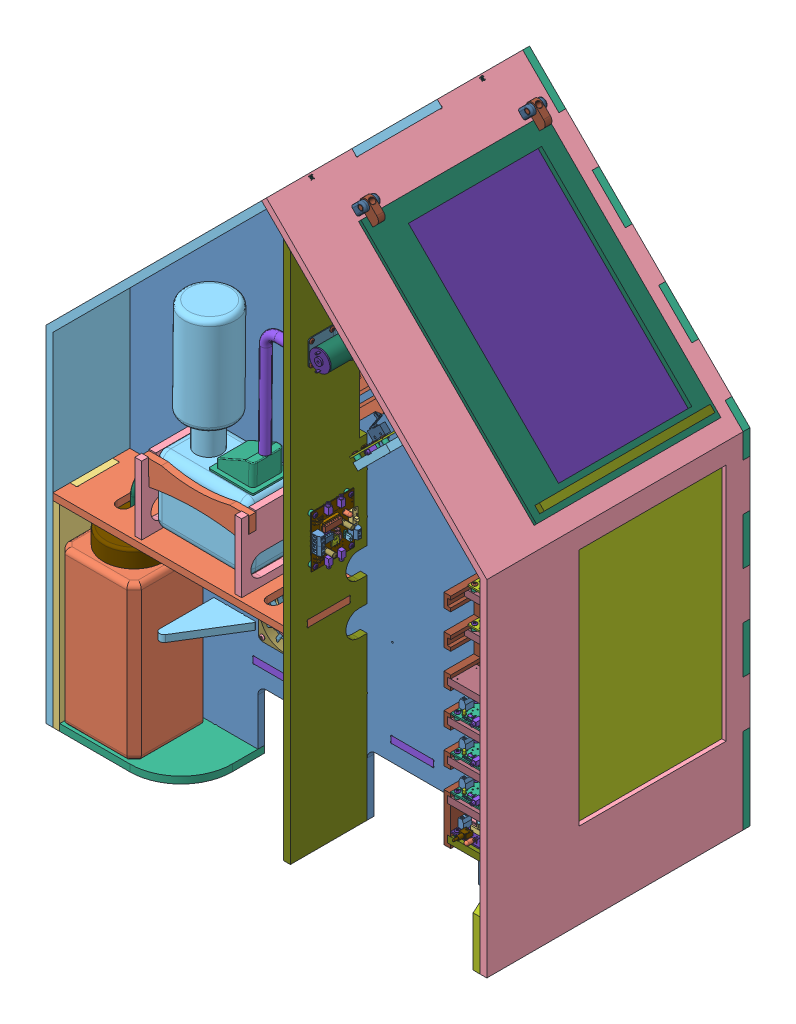
SolidWorks assembly Serre Toutes Options, configuration OLED. Lengths in mm.
Overall size (516 661.85 314.79).
495 component instances, 116 part files, 199 mates.
Components (placement in the parent):
- FONDINTERIEUR-1: FONDINTERIEUR [Défaut] at (-62.876 -300.5478 -4)
- Crémallière M3-3-1: Crémallière M3-3 [Défaut] at (-39.5374 94.1308 4) x (0.707107 0.707107 0) z (0 0 1)
- Rondelle métal 3 x 12-1: Rondelle métal 3 x 12 [Défaut] at (57.939 191.6778 8)
- VIs TC 3 x 13-1: VIs TC 3 x 13 [Défaut] at (57.939 191.6778 2.4) x (1 0 0) z (0 -1 0)
- VIs TC 3 x 13-2: VIs TC 3 x 13 [Défaut] at (22.5836 156.3225 2.4) x (1 0 0) z (0 -1 0)
- Rondelle métal 3 x 12-2: Rondelle métal 3 x 12 [Défaut] at (22.5836 156.3225 8)
- Prépa 06 module Microrupteur-1: Prépa 06 module Microrupteur [Défaut] at (80.8247 148.8026 12.3834) x (0.707107 0.707107 0) z (-0.707107 0.707107 0) size (54 40.91 95.89)
  - support capteur-1: support capteur [Défaut] at (85.4284 22.7312 -4) size (54 38 8)
  - Entretoise CI-1: Entretoise CI [Défaut] at (-25.3985 -17.6166 4) size (5.9 5.9 4.1)
  - Entretoise CI-2: Entretoise CI [Défaut] at (-25.3985 4.3834 4) size (5.9 5.9 4.1)
  - Entretoise CI-3: Entretoise CI [Défaut] at (20.6015 -17.6166 4) size (5.9 5.9 4.1)
  - Entretoise CI-4: Entretoise CI [Défaut] at (20.6015 4.3834 4) size (5.9 5.9 4.1)
  - Module Microrupteur K-AP-MMR-1: Module Microrupteur K-AP-MMR [Défaut] at (24.602 -8.2581 10.6485) x (0 1 0) z (1 0 0) size (32.91 28.24 54)
    - CI-AP-MLBP avec jack-1: CI-AP-MLBP avec jack [Défaut] at (1.5279 -1.3102 0) size (32.91 8.01 54)
      - CI BP et DEL-1: CI BP et DEL [Défaut] at (-14.8869 -1.2382 0) size (30 1.6 54)
      - Embase jack 2.5-1: Embase jack 2.5 [Défaut] at (-14.8868 -1.2382 -27.0002) x (1 0 0) z (0 0 -1) size (10.81 8.01 5)
    - Résistance 10 K pas 11-1: Résistance 10 K pas 11 [Défaut] at (-6.8591 0.4515 -37.4997) x (0 0 -1) z (1 0 0) size (11.5 4.15 2.3)
    - Microrupteur-1: Microrupteur [Défaut] at (16.351 0.0515 -46.78) x (-1 0 0) z (0 0 -1) size (6.3 24.64 22.46)
  - VIs TC 3 x 6.5-1: VIs TC 3 x 6.5 [Défaut] at (-25.3985 -17.6166 3.3) x (1 0 0) z (0 -1 0) size (5.6 8.09 5.6)
  - VIs TC 3 x 6.5-2: VIs TC 3 x 6.5 [Défaut] at (-25.3979 4.3824 3.3) x (1 0 0) z (0 -1 0) size (5.6 8.09 5.6)
  - VIs TC 3 x 6.5-3: VIs TC 3 x 6.5 [Défaut] at (20.6015 -17.6166 3.3) x (0.418214 0.908348 0) z (0.908348 -0.418214 0) size (5.6 8.09 5.6)
  - VIs TC 3 x 6.5-4: VIs TC 3 x 6.5 [Défaut] at (20.6015 4.3834 3.3) x (1 0 0) z (0 -1 0) size (5.6 8.09 5.6)
- Prépa 06 module Microrupteur-2: Prépa 06 module Microrupteur [Défaut] at (10.114 78.0919 12.3834) x (0.707107 0.707107 0) z (-0.707107 0.707107 0) size (54 40.91 95.89)
  - support capteur-1: support capteur [Défaut] at (85.4284 22.7312 -4) size (54 38 8)
  - Entretoise CI-1: Entretoise CI [Défaut] at (-25.3985 -17.6166 4) size (5.9 5.9 4.1)
  - Entretoise CI-2: Entretoise CI [Défaut] at (-25.3985 4.3834 4) size (5.9 5.9 4.1)
  - Entretoise CI-3: Entretoise CI [Défaut] at (20.6015 -17.6166 4) size (5.9 5.9 4.1)
  - Entretoise CI-4: Entretoise CI [Défaut] at (20.6015 4.3834 4) size (5.9 5.9 4.1)
  - Module Microrupteur K-AP-MMR-1: Module Microrupteur K-AP-MMR [Défaut] at (24.602 -8.2581 10.6485) x (0 1 0) z (1 0 0) size (32.91 28.24 54)
    - CI-AP-MLBP avec jack-1: CI-AP-MLBP avec jack [Défaut] at (1.5279 -1.3102 0) size (32.91 8.01 54)
      - CI BP et DEL-1: CI BP et DEL [Défaut] at (-14.8869 -1.2382 0) size (30 1.6 54)
      - Embase jack 2.5-1: Embase jack 2.5 [Défaut] at (-14.8868 -1.2382 -27.0002) x (1 0 0) z (0 0 -1) size (10.81 8.01 5)
    - Résistance 10 K pas 11-1: Résistance 10 K pas 11 [Défaut] at (-6.8591 0.4515 -37.4997) x (0 0 -1) z (1 0 0) size (11.5 4.15 2.3)
    - Microrupteur-1: Microrupteur [Défaut] at (16.351 0.0515 -46.78) x (-1 0 0) z (0 0 -1) size (6.3 24.64 22.46)
  - VIs TC 3 x 6.5-1: VIs TC 3 x 6.5 [Défaut] at (-25.3985 -17.6166 3.3) x (1 0 0) z (0 -1 0) size (5.6 8.09 5.6)
  - VIs TC 3 x 6.5-2: VIs TC 3 x 6.5 [Défaut] at (-25.3979 4.3824 3.3) x (1 0 0) z (0 -1 0) size (5.6 8.09 5.6)
  - VIs TC 3 x 6.5-3: VIs TC 3 x 6.5 [Défaut] at (20.6015 -17.6166 3.3) x (0.418214 0.908348 0) z (0.908348 -0.418214 0) size (5.6 8.09 5.6)
  - VIs TC 3 x 6.5-4: VIs TC 3 x 6.5 [Défaut] at (20.6015 4.3834 3.3) x (1 0 0) z (0 -1 0) size (5.6 8.09 5.6)
- Ventilateur-1: Ventilateur [Défaut] at (-116.5864 -162.967 9.2) size (60 60 10.4)
  - Cage ventilateur-1: Cage ventilateur [Défaut] at (-27.2896 -30.9986 -5.2) size (60 60 10.4)
  - Hélice-1: Hélice [Défaut] at (3.0209 -0.9986 1.3) x (1 0 0) z (0 -1 0) size (55.32 5 55.41)
    - centre hélice-1: centre hélice [Défaut] at (-0.3105 -2.5 0) size (28.6 5 28.6)
    - Pale-1: Pale [Défaut] at (12.924 -1.982 -2.4379) x (-0.128403 0.431224 -0.893061) z (-0.06137 -0.902245 -0.426835) size (5.38 14.29 1.25)
    - Pale-12: Pale [Défaut] at (12.1411 -1.982 5.1043) x (0.374806 0.431224 -0.820711) z (0.179137 -0.902245 -0.392255) size (5.38 14.29 1.25)
    - Pale-13: Pale [Défaut] at (7.4049 -1.982 11.0258) x (0.759017 0.431224 -0.48779) z (0.362769 -0.902245 -0.233137) size (5.38 14.29 1.25)
    - Pale-14: Pale [Défaut] at (0.2191 -1.982 13.4468) x (0.902245 0.431224 0) z (0.431224 -0.902245 0) size (5.38 14.29 1.25)
    - Pale-15: Pale [Défaut] at (-7.1349 -1.982 11.5985) x (0.759017 0.431224 0.48779) z (0.362769 -0.902245 0.233137) size (5.38 14.29 1.25)
    - Pale-16: Pale [Défaut] at (-12.3221 -1.982 6.0677) x (0.374806 0.431224 0.820711) z (0.179137 -0.902245 0.392255) size (5.38 14.29 1.25)
    - Pale-17: Pale [Défaut] at (-13.6958 -1.982 -1.3895) x (-0.128403 0.431224 0.893061) z (-0.06137 -0.902245 0.426835) size (5.38 14.29 1.25)
    - Pale-18: Pale [Défaut] at (-10.8197 -1.982 -8.4055) x (-0.590845 0.431224 0.681871) z (-0.282392 -0.902245 0.325897) size (5.38 14.29 1.25)
    - Pale-19: Pale [Défaut] at (-4.6071 -1.982 -12.7529) x (-0.865698 0.431224 0.254192) z (-0.413756 -0.902245 0.12149) size (5.38 14.29 1.25)
    - Pale-20: Pale [Défaut] at (2.9697 -1.982 -13.0513) x (-0.865698 0.431224 -0.254192) z (-0.413756 -0.902245 -0.12149) size (5.38 14.29 1.25)
    - Pale-21: Pale [Défaut] at (9.505 -1.982 -9.206) x (-0.590845 0.431224 -0.681871) z (-0.282392 -0.902245 -0.325897) size (5.38 14.29 1.25)
- VIs TC 3 x 13-4: VIs TC 3 x 13 [Défaut] at (-138.876 -138.9656 8) x (1 0 0) z (0 -1 0)
- VIs TC 3 x 13-6: VIs TC 3 x 13 [Défaut] at (-88.876 -138.9656 8) x (1 0 0) z (0 -1 0)
- VIs TC 3 x 13-7: VIs TC 3 x 13 [Défaut] at (-88.876 -188.9656 8) x (1 0 0) z (0 -1 0)
- VIs TC 3 x 13-8: VIs TC 3 x 13 [Défaut] at (-138.876 -188.9656 8) x (1 0 0) z (0 -1 0)
- Entretoise CI-1: Entretoise CI [Défaut] at (57.939 191.6778 4) x (-0.97677 0.214292 0) z (0 0 1) size (5.9 5.9 4.1)
- Entretoise CI-2: Entretoise CI [Défaut] at (22.5836 156.3225 4) size (5.9 5.9 4.1)
- VIS TORCX TF 3 X 19-1: VIS TORCX TF 3 X 19 [Défaut] at (79.1287 147.1066 -4) x (-0.923728 -0.383049 0) z (0 0 -1)
- VIS TORCX TF 3 X 19-2: VIS TORCX TF 3 X 19 [Défaut] at (8.418 76.3959 -4) x (-0.923728 -0.383049 0) z (0 0 -1)
- Prépa 02 renfort arrière-1: Prépa 02 renfort arrière [Défaut] at (-30.876 -5.636 -123.7404) x (0 0 -1) z (1 0 0) size (157.27 630.07 217.21)
  - renfortarriere-1: renfortarriere [Défaut] at (-133.6202 -294.9118 -4) size (98 630.07 8)
  - Entretoise CI-1: Entretoise CI [Défaut] at (-194.2138 26.8323 4) size (5.9 5.9 4.1)
  - Entretoise CI-2: Entretoise CI [Défaut] at (-152.2157 27.0837 4) size (5.9 5.9 4.1)
  - Entretoise CI-3: Entretoise CI [Défaut] at (-193.9025 -25.1656 4) size (5.9 5.9 4.1)
  - Entretoise CI-4: Entretoise CI [Défaut] at (-151.9044 -24.9142 4) size (5.9 5.9 4.1)
  - VIs TC 3 x 9-1: VIs TC 3 x 9 [Défaut] at (-194.2138 26.8323 2.7) x (1 0 0) z (0 -1 0) size (5.6 10.69 5.6)
  - VIs TC 3 x 9-2: VIs TC 3 x 9 [Défaut] at (-152.2157 27.0837 2.7) x (1 0 0) z (0 -1 0) size (5.6 10.69 5.6)
  - VIs TC 3 x 9-3: VIs TC 3 x 9 [Défaut] at (-151.9044 -24.9142 2.7) x (1 0 0) z (0 -1 0) size (5.6 10.69 5.6)
  - VIs TC 3 x 9-4: VIs TC 3 x 9 [Défaut] at (-193.9025 -25.1656 2.7) x (1 0 0) z (0 -1 0) size (5.6 10.69 5.6)
  - Module 2 moteurs K-AP-MMOT-1: Module 2 moteurs K-AP-MMOT [Défaut] at (-148.0718 3.1444 10.7771) x (-0.005986 0.999982 0) z (0.999982 0.005986 0) size (65.82 19.5 50.56)
    - CI moteur-1: CI moteur [Défaut] at (-32.0357 -2.6771 0) size (60 1 50)
    - BORNIER 2-1: BORNIER 2 [Default] at (-17.0423 -1.6771 0.2294) x (0.999982 0 0.005986) z (0 1 0) size (9.97 7.55 15.02)
    - DEL D5 R-1: DEL D5 R [Défaut] at (9.6889 6.8229 -10.9906) x (1 0 0) z (0 -1 0) size (5.3 5.6 11.5)
    - Embase jack 2.5-1: Embase jack 2.5 [Défaut] at (-32.0356 -1.6771 -17.5006) size (10.81 8.01 5)
    - MICRO INVERSEUR A GLISSIERE-1: MICRO INVERSEUR A GLISSIERE [Défaut] at (3.55 3.3429 -4.0189) x (1 0 0.000537) z (0 1 0) size (19 5.82 12.15)
    - Résistance 220 ohm pas 11-1: Résistance 220 ohm pas 11 [Défaut] at (-10.0359 0.3229 -18.1991) x (-1 0 0) z (0 0 -1) size (11.5 4.15 2.3)
    - Embase jack 2.5-2: Embase jack 2.5 [Défaut] at (-32.0356 -1.6771 -32.5018) size (10.81 8.01 5)
    - Embase jack 2.5-3: Embase jack 2.5 [Défaut] at (27.964 -1.6771 -17.4981) x (-1 0 0) z (0 0 -1) size (10.81 8.01 5)
    - Embase jack 2.5-4: Embase jack 2.5 [Défaut] at (27.964 -1.6771 -32.4993) x (-1 0 0) z (0 0 -1) size (10.81 8.01 5)
    - Capuchon picot-1: Capuchon picot [Défaut] at (-16.1457 0.4729 -12.7155) x (1 0 0) z (0 -1 0) size (5.05 2.51 6.1)
    - ASB 3PICOTS-1: ASB 3PICOTS [Default] at (-9.9569 2.4259 -10.7946) x (1 0 0) z (0 -1 0) size (7.59 2.51 10)
      - PICOT-1: PICOT [Default] at (26.8516 -23.7306 1.953) size (2.51 2.51 10)
      - PICOT-2: PICOT [Default] at (29.3916 -23.7306 1.953) size (2.51 2.51 10)
      - PICOT-3: PICOT [Default] at (24.3116 -23.7306 1.953) size (2.51 2.51 10)
    - AJUSTABLE H-1: AJUSTABLE H [Défaut] at (-15.4716 0.3229 -24.988) x (0 0 1) z (0 1 0) size (8.6 10.76 7.4)
    - BORNIER 2-2: BORNIER 2 [Default] at (-2.0505 -1.6771 -50.2748) x (-1 0 0) z (0 1 0) size (9.97 7.55 15.02)
    - BORNIER 2-3: BORNIER 2 [Default] at (7.9495 -1.6771 -50.2748) x (-1 0 0) z (0 1 0) size (9.97 7.55 15.02)
    - Résistance 10 K pas 11-1: Résistance 10 K pas 11 [Défaut] at (19.1656 0.3229 -42.727) x (0 0 -1) z (1 0 0) size (11.5 4.15 2.3)
    - Résistance 10 K pas 11-2: Résistance 10 K pas 11 [Défaut] at (15.6274 0.3229 -42.6914) x (0 0 -1) z (1 0 0) size (11.5 4.15 2.3)
    - Résistance 10 K pas 11-3: Résistance 10 K pas 11 [Défaut] at (-19.5364 0.3229 -42.0005) x (0 0 -1) z (1 0 0) size (11.5 4.15 2.3)
    - Résistance 10 K pas 11-4: Résistance 10 K pas 11 [Défaut] at (-23.0365 0.3229 -42.0005) x (0 0 -1) z (1 0 0) size (11.5 4.15 2.3)
    - Support CI 8 pattes-1: Support CI 8 pattes [Défaut] at (-2.7368 -1.6771 -30.0083) x (0 0 -1) z (1 0 0) size (10 6 10.1)
    - Support CI 16 pattes-1: Support CI 16 pattes [Défaut] at (8.6068 -1.6771 -19.8458) x (0 0 -1) z (1 0 0) size (20.1 6 10.1)
    - CI 8 pattes-1: CI 8 pattes [Défaut] at (-2.7368 1.3229 -30.0113) x (0 0 -1) z (1 0 0) size (10 7.2 7.8)
    - CI 16 pattes-1: CI 16 pattes [Défaut] at (8.6068 1.3229 -19.8488) x (0 0 -1) z (1 0 0) size (20.1 7.2 7.8)
    - Capa 16V 100F 2.54-1: Capa 16V 100F 2.54 [Default] at (-14.0347 -26.6935 -37.5006) x (0 0 1) z (-1 0 0) size (5.2 15.5 5.88)
    - Capa 16V 100F 2.54-2: Capa 16V 100F 2.54 [Default] at (2.9618 -26.6935 -15.9995) x (0.999999 0 0.001464) z (-0.001464 0 0.999999) size (5.2 15.5 5.88)
    - condensateur 100nF-1: condensateur 100nF [Default] at (-2.9304 -7.4359 -15.4031) x (0 0 -1) z (1 0 0) size (5.85 10.35 1.99)
    - condensateur 100nF-2: condensateur 100nF [Default] at (0.5738 -7.4359 -15.3738) x (0 0 -1) z (1 0 0) size (5.85 10.35 1.99)
  - Moteur MFA 12-24V-1: Moteur MFA 12-24V [Défaut] at (-181.5572 189.3895 16.5047) x (-1 0 0) z (0 1 0) size (70.4 27.9 30)
    - Support moteur-1: Support moteur [Défaut] at (-14.3868 -12.5047 0) size (31 26.4 30)
    - Corps moteur-1: Corps moteur [Défaut] at (14.8132 1.8953 0) x (0 0 1) z (-1 0 0) size (24 24 63.9)
    - Capuchon moteur-1: Capuchon moteur [Défaut] at (-15.3868 1.8953 0) x (0 0 1) z (-1 0 0) size (27 27 18.7)
    - Arrière moteur-1: Arrière moteur [Défaut] at (16.3132 1.8953 0) x (0 0 1) z (-1 0 0) size (24 24 6.5)
  - Prépa 01 roue dentée-1: Prépa 01 roue dentée [Défaut] at (-131.9704 192.8178 10.3013) x (0 0.156764 -0.987636) z (1 0 0) size (54 54 71.42)
    - roue dentée 16-1: roue dentée 16 [Défaut] at (-7.1573 -1.556 -4) size (54 54 8)
    - Bague d'arrêt 4x12x24-1: Bague d'arrêt 4x12x24 [Défaut] at (-8.536 -2.1164 -10) x (0 1 0) z (0 0 1) size (24 24 8)
    - VIs TC 3 x 6.5-1: VIs TC 3 x 6.5 [Défaut] at (-8.536 6.8836 2.4) x (1 0 0) z (0 1 0) size (5.6 8.09 5.6)
    - VIs TC 3 x 6.5-2: VIs TC 3 x 6.5 [Défaut] at (-8.536 -11.1164 2.4) x (1 0 0) z (0 1 0) size (5.6 8.09 5.6)
  - VIs TC 3 x 6.5-1: VIs TC 3 x 6.5 [Défaut] at (-194.1704 201.3895 -1.4) x (1 0 0) z (0 -1 0) size (5.6 8.09 5.6)
  - VIs TC 3 x 6.5-2: VIs TC 3 x 6.5 [Défaut] at (-170.1704 201.3895 -1.4) x (1 0 0) z (0 -1 0) size (5.6 8.09 5.6)
  - VIs TC 3 x 6.5-3: VIs TC 3 x 6.5 [Défaut] at (-194.1704 177.3895 -1.4) x (1 0 0) z (0 -1 0) size (5.6 8.09 5.6)
  - VIs TC 3 x 6.5-4: VIs TC 3 x 6.5 [Défaut] at (-170.1704 177.3895 -1.4) x (1 0 0) z (0 -1 0) size (5.6 8.09 5.6)
- étagèrebrumi-1: étagèrebrumi [Défaut] at (-62.876 -93.9656 245.3364) x (1 0 0) z (0 1 0)
- VIS TORCX TF 3 X 19-3: VIS TORCX TF 3 X 19 [Défaut] at (-30.876 -315.9656 -4) x (-0.991079 -0.133274 0) z (0 0 -1)
- VIS TORCX TF 3 X 19-4: VIS TORCX TF 3 X 19 [Défaut] at (-30.876 -274.5499 -4) x (-0.991079 -0.133274 0) z (0 0 -1)
- VIS TORCX TF 3 X 19-5: VIS TORCX TF 3 X 19 [Défaut] at (-169.876 -89.9656 -4) x (-0.991079 -0.133274 0) z (0 0 -1)
- VIS TORCX TF 3 X 19-6: VIS TORCX TF 3 X 19 [Défaut] at (-30.876 -27.0369 -4) x (-0.991079 -0.133274 0) z (0 0 -1)
- VIS TORCX TF 3 X 19-7: VIS TORCX TF 3 X 19 [Défaut] at (-30.876 278.5344 -4) x (-0.991079 -0.133274 0) z (0 0 -1)
- Coté gauche serre-1: Coté gauche serre [Défaut] at (-304.876 -288.0405 43.9648) x (0 0 -1) z (1 0 0)
- Coté support brumisateur-1: Coté support brumisateur [Défaut] at (-87.876 -76.5368 52.2063) x (0 0 1) z (-1 0 0)
- Coté support brumisateur-2: Coté support brumisateur [Défaut] at (-204.876 -76.5368 52.2063) x (0 0 1) z (-1 0 0)
- Renfort bidon-1: Renfort bidon [Défaut] at (-206.376 -195.9656 85) x (1 0 0) z (0 1 0)
- suportbloceau-1: suportbloceau [Défaut] at (-238.3888 -323.9656 72.4161) x (1 0 0) z (0 1 0)
- VIS TORCX TF 3 X 19-12: VIS TORCX TF 3 X 19 [Défaut] at (-198.876 -191.9656 -4) x (-0.923728 -0.383049 0) z (0 0 -1)
- VIS TORCX TF 3 X 19-13: VIS TORCX TF 3 X 19 [Défaut] at (-164.4919 -191.9656 -4) x (-0.923728 -0.383049 0) z (0 0 -1)
- VIS TORCX TF 3 X 19-14: VIS TORCX TF 3 X 19 [Défaut] at (-208.876 -75.9656 -4) x (-0.923728 -0.383049 0) z (0 0 -1)
- VIS TORCX TF 3 X 19-15: VIS TORCX TF 3 X 19 [Défaut] at (-208.876 -16.4656 -4) x (-0.923728 -0.383049 0) z (0 0 -1)
- VIS TORCX TF 3 X 19-16: VIS TORCX TF 3 X 19 [Défaut] at (-91.876 -75.9656 -4) x (-0.923728 -0.383049 0) z (0 0 -1)
- VIS TORCX TF 3 X 19-17: VIS TORCX TF 3 X 19 [Défaut] at (-91.876 -15.9656 -4) x (-0.923728 -0.383049 0) z (0 0 -1)
- VIS TORCX TF 3 X 19-18: VIS TORCX TF 3 X 19 [Défaut] at (-304.876 -89.9656 48.9996) x (0 0 1) z (-1 0 0)
- VIS TORCX TF 3 X 19-25: VIS TORCX TF 3 X 19 [Défaut] at (-304.876 -248.9656 -0.0009) x (0 0 1) z (-1 0 0)
- VIS TORCX TF 3 X 19-26: VIS TORCX TF 3 X 19 [Défaut] at (-300.876 -323.9656 49) x (0.782535 0 -0.622606) z (0 -1 0)
- VIS TORCX TF 3 X 19-29: VIS TORCX TF 3 X 19 [Défaut] at (-271.876 -323.9656 0) x (0.782535 0 -0.622606) z (0 -1 0)
- VIS TORCX TF 3 X 19-30: VIS TORCX TF 3 X 19 [Défaut] at (-179.876 -323.9656 0) x (0.782535 0 -0.622606) z (0 -1 0)
- Coté droit serre-1: Coté droit serre [Défaut] at (187.124 -288.4466 43.9657) x (0 0 -1) z (1 0 0)
- VIS TORCX TF 3 X 19-35: VIS TORCX TF 3 X 19 [Défaut] at (195.124 -248.9656 0) x (0 -0.192039 -0.981387) z (1 0 0)
- Poutre fond-1: Poutre fond [Défaut] at (-62.876 -231.9656 64.5822) x (1 0 0) z (0 1 0)
- VIS TORCX TF 3 X 19-36: VIS TORCX TF 3 X 19 [Défaut] at (-213.1345 -227.9656 4)
- VIS TORCX TF 3 X 19-37: VIS TORCX TF 3 X 19 [Défaut] at (-54.876 -227.9656 4)
- Poutre plateau-1: Poutre plateau [Défaut] at (79.7388 -229.6404 -13) x (-1 0 0) z (0 0 -1)
- façadeporteplateau-1: façadeporteplateau [Défaut] at (102.5126 -276.3164 -206)
- VIS TORCX TF 3 X 19-38: VIS TORCX TF 3 X 19 [Défaut] at (191.124 -273.9656 -206) x (-0.923728 -0.383049 0) z (0 0 -1)
- VIS TORCX TF 3 X 19-39: VIS TORCX TF 3 X 19 [Défaut] at (195.124 -308.9656 -202) x (0 0 -1) z (1 0 0)
- VIS TORCX TF 3 X 19-40: VIS TORCX TF 3 X 19 [Défaut] at (195.124 -238.9656 -202) x (0 0 -1) z (1 0 0)
- VIS TORCX TF 3 X 19-43: VIS TORCX TF 3 X 19 [Défaut] at (-300.876 -273.9656 -206) x (-0.923728 -0.383049 0) z (0 0 -1)
- VIS TORCX TF 3 X 19-44: VIS TORCX TF 3 X 19 [Défaut] at (-304.876 -238.9737 -202) x (0 0 1) z (-1 0 0)
- VIS TORCX TF 3 X 19-45: VIS TORCX TF 3 X 19 [Défaut] at (-304.876 -308.9656 -202) x (0 0 1) z (-1 0 0)
- VIS TORCX TF 3 X 19-49: VIS TORCX TF 3 X 19 [Défaut] at (103.3825 -227.9656 4)
- Sous ensemble Rack module Toutes Options-1: Sous ensemble Rack module Toutes Options [Défaut] at (116.8547 -126.3174 -67.6389) x (0 0 -1) z (1 0 0) size (72.22 263.1 70)
  - rack coté gauche-1: rack coté gauche [Défaut] at (-102.2159 -95.6801 -4) size (58 256 8)
  - rack coté droit-1: rack coté droit [Défaut] at (-102.2159 -95.6628 58) size (58 256 8)
  - Prépa 05 module TEMP-1: Prépa 05 module TEMP [Défaut] at (-82.7846 122.513 33.0896) x (0 0 1) z (0 1 0) size (62 41.41 95.55)
    - supportcarterack-1: supportcarterack [Défaut] at (3.5074 9.0286 -6.1612) size (62 30 8)
    - Entretoise CI-1: Entretoise CI [Défaut] at (-25.0896 -14.8542 1.8388) size (5.9 5.9 4.1)
    - Entretoise CI-2: Entretoise CI [Défaut] at (-25.0896 7.1458 1.8388) size (5.9 5.9 4.1)
    - Entretoise CI-3: Entretoise CI [Défaut] at (20.9104 -14.8542 1.8388) size (5.9 5.9 4.1)
    - Entretoise CI-4: Entretoise CI [Défaut] at (20.9104 7.1458 1.8388) size (5.9 5.9 4.1)
    - Module temperature K-AP-MTEMP-1: Module temperature K-AP-MTEMP [Défaut] at (24.9109 -3.9678 7.1771) x (0 1 0) z (1 0 0) size (41.41 8.39 54)
      - CI BP et DEL-1: CI BP et DEL [Défaut] at (-14.8869 -1.2382 0) size (30 1.6 54)
      - Embase jack 2.5-1: Embase jack 2.5 [Défaut] at (-14.8868 0.3618 -27.0002) size (10.81 8.01 5)
      - Résistance 3,9 K pas 11-1: Résistance 3,9 K pas 11 [Défaut] at (-12.3875 1.7618 -37.4997) x (0 0 1) z (-1 0 0) size (11.5 4.15 2.3)
      - RC1 Tansistor plié 90°-1: RC1 Tansistor plié 90° [Défaut] at (18.6119 3.3399 -22.4989) x (0 0 -1) z (0 -1 0) size (4.8 10.25 6.98)
    - VIs TC 3 x 6.5-1: VIs TC 3 x 6.5 [Défaut] at (-25.0896 -14.8542 1.1388) x (1 0 0) z (0 -1 0) size (5.6 8.09 5.6)
    - VIs TC 3 x 6.5-2: VIs TC 3 x 6.5 [Défaut] at (-25.0896 7.1458 1.1388) x (1 0 0) z (0 -1 0) size (5.6 8.09 5.6)
    - VIs TC 3 x 6.5-3: VIs TC 3 x 6.5 [Défaut] at (20.9104 7.1458 1.1388) x (1 0 0) z (0 -1 0) size (5.6 8.09 5.6)
    - VIs TC 3 x 6.5-4: VIs TC 3 x 6.5 [Défaut] at (20.9104 -14.8542 1.1388) x (1 0 0) z (0 -1 0) size (5.6 8.09 5.6)
  - VIS TORCX TF 3 X 19-1: VIS TORCX TF 3 X 19 [Défaut] at (-86.6389 120.3518 66)
  - VIS TORCX TF 3 X 19-2: VIS TORCX TF 3 X 19 [Défaut] at (-86.6389 120.3431 -4) x (-0.923728 -0.383049 0) z (0 0 -1)
  - Prépa 04 module MAFU-1: Prépa 04 module MAFU [Défaut] at (-94.8752 -119.6656 28.2245) x (0 0 1) z (0 1 0) size (62 61.57 131.04)
    - basesuportpuissance-1: basesuportpuissance [Défaut] at (-4.8343 -1.5394 -4) size (62 50 8)
    - Entretoise CI-1: Entretoise CI [Défaut] at (-20.2245 -22.7636 4) size (5.9 5.9 4.1)
    - Entretoise CI-2: Entretoise CI [Défaut] at (-20.2245 -0.7636 4) size (5.9 5.9 4.1)
    - Entretoise CI-3: Entretoise CI [Défaut] at (25.7755 -0.7636 4) size (5.9 5.9 4.1)
    - Entretoise CI-4: Entretoise CI [Défaut] at (25.7755 -22.7636 4) size (5.9 5.9 4.1)
    - CI-MAFU avec borniers-1: CI-MAFU avec borniers [Défaut] at (2.9088 -18.7288 8.9) x (0 -1 0) z (0 0 1) size (43.65 55.05 18.42)
      - CI-MAFU-1: CI-MAFU [Défaut] at (-21.9652 -27.1333 -0.8) size (30 54 1.6)
      - Inter long à souder 734-7220-1: Inter long à souder 734-7220 [Défaut] at (8.1051 -9.1203 1.3) x (-1 0 0) z (0 1 0) size (20.8 9.2 8)
      - Embase femelle d'alimentation-1: Embase femelle d'alimentation [Défaut] at (4.7338 12.8853 0.8) x (0 -1 0) z (-1 0 0) size (10.39 15 14.1)
      - DEL D5 rouge pliée-2: DEL D5 rouge pliée [Défaut] at (17.5325 -1.131 5.2) x (0 1 0) z (-1 0 0) size (5.3 8.8 12.9)
      - Support fusible avec fusible-1: Support fusible avec fusible [Défaut] at (-8.3615 -5.1853 4.8987) x (0 1 0) z (1 0 0) size (23 17 8.6)
        - Support fusible base-1: Support fusible base [Défaut] at (-10.9359 -4.0987 -4.3) size (22 7 8.6)
        - Support fusible contact-1: Support fusible contact [Défaut] at (5.4641 0.8731 -0.0014) size (6.1 17 6.2)
        - Support fusible contact-2: Support fusible contact [Défaut] at (-5.3359 0.8731 -0.0014) x (-1 0 0) z (0 0 -1) size (6.1 17 6.2)
        - Fusible-1: Fusible [Défaut] at (-0.0359 6.2731 -0.0014) size (19.8 5.2 5.2)
      - BORNIER 2-2: BORNIER 2 [Default] at (-24.0402 -10.1483 0.8) x (0 -1 0) z (0 0 1) size (9.97 7.55 15.02)
      - BORNIER 2-4: BORNIER 2 [Default] at (-24.0402 -0.1483 0.8) x (0 -1 0) z (0 0 1) size (9.97 7.55 15.02)
      - BORNIER 2-5: BORNIER 2 [Default] at (-24.0402 9.8517 0.8) x (0 -1 0) z (0 0 1) size (9.97 7.55 15.02)
      - BORNIER 2-6: BORNIER 2 [Default] at (-24.0402 19.8517 0.8) x (0 -1 0) z (0 0 1) size (9.97 7.55 15.02)
      - BORNIER 2-7: BORNIER 2 [Default] at (-10.2502 -27.9083 0.8) size (9.97 7.55 15.02)
      - BORNIER 2-9: BORNIER 2 [Default] at (-0.2802 27.1417 0.8) x (-1 0 0) z (0 0 1) size (9.97 7.55 15.02) (hidden)
    - VIs TC 3 x 9-1: VIs TC 3 x 9 [Défaut] at (-20.2245 -22.7636 3.3) x (1 0 0) z (0 -1 0) size (5.6 10.69 5.6)
    - VIs TC 3 x 9-2: VIs TC 3 x 9 [Défaut] at (25.7755 -22.7636 3.3) x (1 0 0) z (0 -1 0) size (5.6 10.69 5.6)
    - VIs TC 3 x 9-3: VIs TC 3 x 9 [Défaut] at (-20.2245 -0.7636 3.3) x (1 0 0) z (0 -1 0) size (5.6 10.69 5.6)
    - VIs TC 3 x 9-4: VIs TC 3 x 9 [Défaut] at (25.7755 -0.7636 3.3) x (1 0 0) z (0 -1 0) size (5.6 10.69 5.6)
  - VIS TORCX TF 3 X 19-3: VIS TORCX TF 3 X 19 [Défaut] at (-107.1389 -119.6824 66)
  - VIS TORCX TF 3 X 19-4: VIS TORCX TF 3 X 19 [Défaut] at (-78.1389 -119.6824 66)
  - VIS TORCX TF 3 X 19-6: VIS TORCX TF 3 X 19 [Défaut] at (-107.1389 -119.6656 -4) x (-0.923728 -0.383049 0) z (0 0 -1)
  - VIS TORCX TF 3 X 19-7: VIS TORCX TF 3 X 19 [Défaut] at (-78.1389 -119.6656 -4) x (-0.923728 -0.383049 0) z (0 0 -1)
  - Prépa 03 module PWR-1: Prépa 03 module PWR [Défaut] at (-104.636 -79.6656 32.1892) x (0 0 1) z (0 1 0) size (62 33.06 100.16)
    - supportcarterack-1: supportcarterack [Défaut] at (4.4079 10.88 -4) size (62 30 8)
    - Entretoise CI-1: Entretoise CI [Défaut] at (-24.1892 -13.0028 4) size (5.9 5.9 4.1)
    - Entretoise CI-2: Entretoise CI [Défaut] at (-24.1892 8.9972 4) size (5.9 5.9 4.1)
    - Entretoise CI-3: Entretoise CI [Défaut] at (21.8108 8.9972 4) size (5.9 5.9 4.1)
    - Entretoise CI-4: Entretoise CI [Défaut] at (21.8108 -13.0028 4) size (5.9 5.9 4.1)
    - Module K-AP-MPWR-1: Module K-AP-MPWR [Défaut] at (-1.2571 1.9363 8.9) x (0 1 0) z (0 0 1) size (33.06 54.47 15.02)
      - CI AP-PWR-1: CI AP-PWR [Défaut] at (-18.9391 -27.0679 -0.8) size (30 54 1.6)
      - BORNIER 2-1: BORNIER 2 [Default] at (0.963 27.1235 0.8) x (-1 0 0) z (0 0 1) size (9.97 7.55 15.02)
      - DELverte 3mm-1: DELverte 3mm [Défaut] at (-12.9358 16.93 1.8) x (0 0 1) z (-1 0 0) size (7.4 3.42 3.8)
      - diode-1: diode [Défaut] at (-12.9396 11.4315 3.2) x (1 0 0) z (0 -1 0) size (2.65 5.32 8.12)
      - ASB 3PICOTS avec capuchon-1: ASB 3PICOTS avec capuchon [Default] at (-16.084 -16.9024 4.903) x (-1 0 0) z (0 0 -1) size (7.59 2.51 10.25)
        - PICOT-1: PICOT [Default] at (26.8516 -23.7306 1.953) size (2.51 2.51 10)
        - PICOT-2: PICOT [Default] at (29.3916 -23.7306 1.953) size (2.51 2.51 10)
        - PICOT-3: PICOT [Default] at (24.3116 -23.7306 1.953) size (2.51 2.51 10)
        - Capuchon picot-1: Capuchon picot [Défaut] at (-6.1888 -1.9209 1.953) size (5.05 2.51 6.1)
      - Embase jack 2.5-1: Embase jack 2.5 [Défaut] at (-18.9403 -0.0677 0.8) x (1 0 0) z (0 -1 0) size (10.81 8.01 5)
      - REG-1: REG [Default] at (-4.2884 5.0073 0.8) x (0 -1 0) z (0 0 1) size (10.15 20.05 5.19)
      - Résistance 220 pas 11-1: Résistance 220 pas 11 [Défaut] at (-17.2386 9.3312 2.2) x (0 -1 0) z (-1 0 0) size (11.5 4.15 2.3)
      - Résistance 10K pas de 11-1: Résistance 10K pas de 11 [Défaut] at (-17.2386 -9.3683 2.2) x (0 -1 0) z (-1 0 0) size (11.5 4.15 2.3)
      - BORNIER 2-2: BORNIER 2 [Default] at (-8.9238 -27.3428 0.8) size (9.97 7.55 15.02)
    - VIs TC 3 x 9-1: VIs TC 3 x 9 [Défaut] at (-24.1892 -13.0028 3.3) x (1 0 0) z (0 -1 0) size (5.6 10.69 5.6)
    - VIs TC 3 x 9-2: VIs TC 3 x 9 [Défaut] at (-24.1892 8.9972 3.3) x (1 0 0) z (0 -1 0) size (5.6 10.69 5.6)
    - VIs TC 3 x 9-3: VIs TC 3 x 9 [Défaut] at (21.8108 8.9972 3.3) x (1 0 0) z (0 -1 0) size (5.6 10.69 5.6)
    - VIs TC 3 x 9-4: VIs TC 3 x 9 [Défaut] at (21.8108 -13.0028 3.3) x (1 0 0) z (0 -1 0) size (5.6 10.69 5.6)
  - supportcarterack-3: supportcarterack [Défaut] at (-119.5217 44.3518 36.597) x (0 0 1) z (0 -1 0) size (62 30 8)
  - Prépa 03 module PWR-2: Prépa 03 module PWR [Défaut] at (-104.636 -39.6656 32.1892) x (0 0 1) z (0 1 0) size (62 33.06 100.16)
    - supportcarterack-1: supportcarterack [Défaut] at (4.4079 10.88 -4) size (62 30 8)
    - Entretoise CI-1: Entretoise CI [Défaut] at (-24.1892 -13.0028 4) size (5.9 5.9 4.1)
    - Entretoise CI-2: Entretoise CI [Défaut] at (-24.1892 8.9972 4) size (5.9 5.9 4.1)
    - Entretoise CI-3: Entretoise CI [Défaut] at (21.8108 8.9972 4) size (5.9 5.9 4.1)
    - Entretoise CI-4: Entretoise CI [Défaut] at (21.8108 -13.0028 4) size (5.9 5.9 4.1)
    - Module K-AP-MPWR-1: Module K-AP-MPWR [Défaut] at (-1.2571 1.9363 8.9) x (0 1 0) z (0 0 1) size (33.06 54.47 15.02)
      - CI AP-PWR-1: CI AP-PWR [Défaut] at (-18.9391 -27.0679 -0.8) size (30 54 1.6)
      - BORNIER 2-1: BORNIER 2 [Default] at (0.963 27.1235 0.8) x (-1 0 0) z (0 0 1) size (9.97 7.55 15.02)
      - DELverte 3mm-1: DELverte 3mm [Défaut] at (-12.9358 16.93 1.8) x (0 0 1) z (-1 0 0) size (7.4 3.42 3.8)
      - diode-1: diode [Défaut] at (-12.9396 11.4315 3.2) x (1 0 0) z (0 -1 0) size (2.65 5.32 8.12)
      - ASB 3PICOTS avec capuchon-1: ASB 3PICOTS avec capuchon [Default] at (-16.084 -16.9024 4.903) x (-1 0 0) z (0 0 -1) size (7.59 2.51 10.25)
        - PICOT-1: PICOT [Default] at (26.8516 -23.7306 1.953) size (2.51 2.51 10)
        - PICOT-2: PICOT [Default] at (29.3916 -23.7306 1.953) size (2.51 2.51 10)
        - PICOT-3: PICOT [Default] at (24.3116 -23.7306 1.953) size (2.51 2.51 10)
        - Capuchon picot-1: Capuchon picot [Défaut] at (-6.1888 -1.9209 1.953) size (5.05 2.51 6.1)
      - Embase jack 2.5-1: Embase jack 2.5 [Défaut] at (-18.9403 -0.0677 0.8) x (1 0 0) z (0 -1 0) size (10.81 8.01 5)
      - REG-1: REG [Default] at (-4.2884 5.0073 0.8) x (0 -1 0) z (0 0 1) size (10.15 20.05 5.19)
      - Résistance 220 pas 11-1: Résistance 220 pas 11 [Défaut] at (-17.2386 9.3312 2.2) x (0 -1 0) z (-1 0 0) size (11.5 4.15 2.3)
      - Résistance 10K pas de 11-1: Résistance 10K pas de 11 [Défaut] at (-17.2386 -9.3683 2.2) x (0 -1 0) z (-1 0 0) size (11.5 4.15 2.3)
      - BORNIER 2-2: BORNIER 2 [Default] at (-8.9238 -27.3428 0.8) size (9.97 7.55 15.02)
    - VIs TC 3 x 9-1: VIs TC 3 x 9 [Défaut] at (-24.1892 -13.0028 3.3) x (1 0 0) z (0 -1 0) size (5.6 10.69 5.6)
    - VIs TC 3 x 9-2: VIs TC 3 x 9 [Défaut] at (-24.1892 8.9972 3.3) x (1 0 0) z (0 -1 0) size (5.6 10.69 5.6)
    - VIs TC 3 x 9-3: VIs TC 3 x 9 [Défaut] at (21.8108 8.9972 3.3) x (1 0 0) z (0 -1 0) size (5.6 10.69 5.6)
    - VIs TC 3 x 9-4: VIs TC 3 x 9 [Défaut] at (21.8108 -13.0028 3.3) x (1 0 0) z (0 -1 0) size (5.6 10.69 5.6)
  - Prépa 03 module PWR-3: Prépa 03 module PWR [Défaut] at (-104.636 0.3344 32.1892) x (0 0 1) z (0 1 0) size (62 33.06 100.16)
    - supportcarterack-1: supportcarterack [Défaut] at (4.4079 10.88 -4) size (62 30 8)
    - Entretoise CI-1: Entretoise CI [Défaut] at (-24.1892 -13.0028 4) size (5.9 5.9 4.1)
    - Entretoise CI-2: Entretoise CI [Défaut] at (-24.1892 8.9972 4) size (5.9 5.9 4.1)
    - Entretoise CI-3: Entretoise CI [Défaut] at (21.8108 8.9972 4) size (5.9 5.9 4.1)
    - Entretoise CI-4: Entretoise CI [Défaut] at (21.8108 -13.0028 4) size (5.9 5.9 4.1)
    - Module K-AP-MPWR-1: Module K-AP-MPWR [Défaut] at (-1.2571 1.9363 8.9) x (0 1 0) z (0 0 1) size (33.06 54.47 15.02)
      - CI AP-PWR-1: CI AP-PWR [Défaut] at (-18.9391 -27.0679 -0.8) size (30 54 1.6)
      - BORNIER 2-1: BORNIER 2 [Default] at (0.963 27.1235 0.8) x (-1 0 0) z (0 0 1) size (9.97 7.55 15.02)
      - DELverte 3mm-1: DELverte 3mm [Défaut] at (-12.9358 16.93 1.8) x (0 0 1) z (-1 0 0) size (7.4 3.42 3.8)
      - diode-1: diode [Défaut] at (-12.9396 11.4315 3.2) x (1 0 0) z (0 -1 0) size (2.65 5.32 8.12)
      - ASB 3PICOTS avec capuchon-1: ASB 3PICOTS avec capuchon [Default] at (-16.084 -16.9024 4.903) x (-1 0 0) z (0 0 -1) size (7.59 2.51 10.25)
        - PICOT-1: PICOT [Default] at (26.8516 -23.7306 1.953) size (2.51 2.51 10)
        - PICOT-2: PICOT [Default] at (29.3916 -23.7306 1.953) size (2.51 2.51 10)
        - PICOT-3: PICOT [Default] at (24.3116 -23.7306 1.953) size (2.51 2.51 10)
        - Capuchon picot-1: Capuchon picot [Défaut] at (-6.1888 -1.9209 1.953) size (5.05 2.51 6.1)
      - Embase jack 2.5-1: Embase jack 2.5 [Défaut] at (-18.9403 -0.0677 0.8) x (1 0 0) z (0 -1 0) size (10.81 8.01 5)
      - REG-1: REG [Default] at (-4.2884 5.0073 0.8) x (0 -1 0) z (0 0 1) size (10.15 20.05 5.19)
      - Résistance 220 pas 11-1: Résistance 220 pas 11 [Défaut] at (-17.2386 9.3312 2.2) x (0 -1 0) z (-1 0 0) size (11.5 4.15 2.3)
      - Résistance 10K pas de 11-1: Résistance 10K pas de 11 [Défaut] at (-17.2386 -9.3683 2.2) x (0 -1 0) z (-1 0 0) size (11.5 4.15 2.3)
      - BORNIER 2-2: BORNIER 2 [Default] at (-8.9238 -27.3428 0.8) size (9.97 7.55 15.02)
    - VIs TC 3 x 9-1: VIs TC 3 x 9 [Défaut] at (-24.1892 -13.0028 3.3) x (1 0 0) z (0 -1 0) size (5.6 10.69 5.6)
    - VIs TC 3 x 9-2: VIs TC 3 x 9 [Défaut] at (-24.1892 8.9972 3.3) x (1 0 0) z (0 -1 0) size (5.6 10.69 5.6)
    - VIs TC 3 x 9-3: VIs TC 3 x 9 [Défaut] at (21.8108 8.9972 3.3) x (1 0 0) z (0 -1 0) size (5.6 10.69 5.6)
    - VIs TC 3 x 9-4: VIs TC 3 x 9 [Défaut] at (21.8108 -13.0028 3.3) x (1 0 0) z (0 -1 0) size (5.6 10.69 5.6)
  - Prépa 07 module Humidité-1: Prépa 07 module Humidité [Défaut] at (-82.3194 80.3344 31.1565) x (0 0 1) z (0 1 0) size (62 43.56 18.7)
    - supportcarterack-1: supportcarterack [Défaut] at (5.4405 8.5634 -4) size (62 30 8)
    - Entretoise CI-1: Entretoise CI [Défaut] at (-23.1565 -15.3194 4) size (5.9 5.9 4.1)
    - Entretoise CI-2: Entretoise CI [Défaut] at (-23.1565 6.6806 4) size (5.9 5.9 4.1)
    - Entretoise CI-3: Entretoise CI [Défaut] at (22.8435 -15.3194 4) size (5.9 5.9 4.1)
    - Entretoise CI-4: Entretoise CI [Défaut] at (22.8435 6.6806 4) size (5.9 5.9 4.1)
    - Carte M-HUM-1: Carte M-HUM [Défaut] at (26.844 -4.433 9.3382) x (0 1 0) z (1 0 0) size (43.56 8.01 54)
      - CI BP et DEL-1: CI BP et DEL [Défaut] at (-14.8869 -1.2382 0) size (30 1.6 54)
      - Embase jack 2.5-1: Embase jack 2.5 [Défaut] at (-14.8868 0.3618 -27.0002) size (10.81 8.01 5)
      - Résistance 150 k pas 11-1: Résistance 150 k pas 11 [Défaut] at (0.1131 1.7618 -35.4025) size (11.5 4.15 2.3)
      - Capteur Humidité-1: Capteur Humidité [Défaut] at (17.138 2.3618 -12.6924) x (-0.0095 0 0.999955) z (-0.999955 0 -0.0095) size (5.67 5.6 13.21)
    - VIs TC 3 x 9-1: VIs TC 3 x 9 [Défaut] at (-23.1565 -15.3194 3.3) x (1 0 0) z (0 -1 0) size (5.6 10.69 5.6)
    - VIs TC 3 x 9-2: VIs TC 3 x 9 [Défaut] at (-23.1559 6.6795 3.3) x (1 0 0) z (0 -1 0) size (5.6 10.69 5.6)
    - VIs TC 3 x 9-3: VIs TC 3 x 9 [Défaut] at (22.8435 -15.3194 3.3) x (1 0 0) z (0 -1 0) size (5.6 10.69 5.6)
    - VIs TC 3 x 9-4: VIs TC 3 x 9 [Défaut] at (22.8435 6.6795 3.3) x (1 0 0) z (0 -1 0) size (5.6 10.69 5.6)
